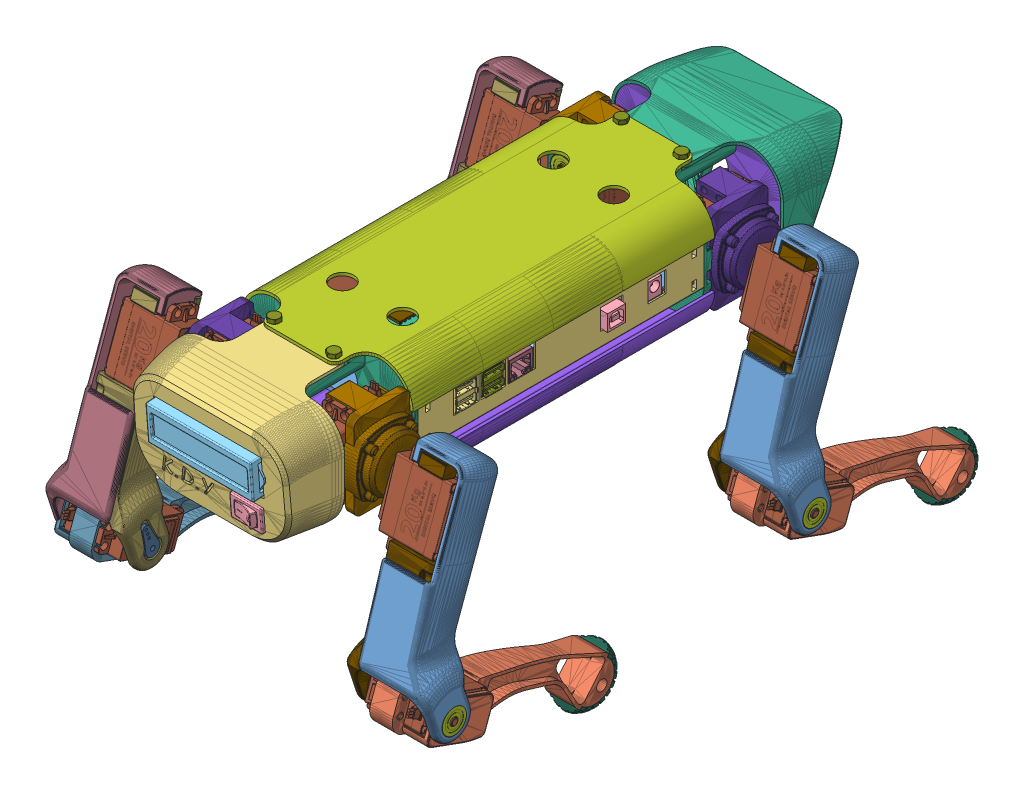
SolidWorks assembly Full Assembly [regular legs], configuration Default. Lengths in mm.
Overall size (257.32 212.52 418.73).
208 component instances, 46 part files, 86 mates.
Components (placement in the parent):
- Chase Assembly-1: Chase Assembly [Default] at (121.4756 142.8431 224.0299) size (112.8 70 292)
  - 1_2MCU_Plate-1: 1_2MCU_Plate [Default] at (22.3647 94.0168 229.1495) size (106 5.81 180)
  - 2_2MCU_Left_side_plate-1: 2_2MCU_Left_side_plate [Default] at (18.1147 57.0168 99.1495) x (1 0 0) z (0 -1 0) size (6.5 190 29)
  - 3_2MCU_Right_side_plate-1: 3_2MCU_Right_side_plate [Default] at (121.6147 57.0168 169.1495) x (-1 0 0) z (0 -1 0) size (6.5 190 29)
  - ArduinoMega-1: ArduinoMega [Default] at (70.5126 101.4678 88.5891) x (1 0 0) z (0 -1 0) size (107.95 53.42 12.95)
  - _Hex_Screws-1: _Hex_Screws [H M3x8] at (55.5647 101.4678 97.3157) x (-0.837169 0 -0.546944) z (-0.546944 0 0.837169) size (5.5 10 6.35) (hidden)
  - _Hex_Screws-2: _Hex_Screws [H M3x8] at (55.5647 101.4678 69.2995) x (0.837169 0 0.546944) z (0.546944 0 -0.837169) size (5.5 10 6.35) (hidden)
  - 4_M3_nut-1: 4_M3_nut [Default] at (55.5655 95.0168 69.2614) x (0.855198 0 0.518302) z (-0.518302 0 0.855198) size (6 2.34 5.2) (hidden)
  - 4_M3_nut-2: 4_M3_nut [Default] at (55.5332 95.0168 97.2415) x (-0.878773 0 0.47724) z (-0.47724 0 -0.878773) size (6 2.34 5.2) (hidden)
  - 12Channel PWM-1: 12Channel PWM [Default] at (79.9147 99.8168 132.7995) x (0 0 -1) z (1 0 0) size (25.4 7.55 66.7)
  - _M2_nut-1: _M2_nut [Default] at (51.9456 95.5168 142.2881) x (-0.74075 0 -0.671781) z (0 -1 0) size (4.67 4.62 1.63) (hidden)
  - _M2_nut-2: _M2_nut [Default] at (107.8452 93.9168 142.288) x (-0.738205 0 -0.674577) z (0 1 0) size (4.67 4.62 1.63) (hidden)
  - _M2_nut-3: _M2_nut [Default] at (107.8453 93.9168 123.488) x (-0.739008 0 -0.673697) z (0 1 0) size (4.67 4.62 1.63) (hidden)
  - _M2_nut-4: _M2_nut [Default] at (51.8785 93.9168 123.4273) x (-0.741456 0 -0.671001) z (0 1 0) size (4.67 4.62 1.63) (hidden)
  - _Hex_Screws-3: _Hex_Screws [H M2x8] at (51.9647 101.3268 142.1995) x (0.837169 0 0.546944) z (0.546944 0 -0.837169) size (4 9.4 4.62) (hidden)
  - _Hex_Screws-4: _Hex_Screws [H M2x8] at (107.8647 101.3268 123.3995) x (0.837169 0 0.546944) z (0.546944 0 -0.837169) size (4 9.4 4.62) (hidden)
  - _Hex_Screws-5: _Hex_Screws [H M2x8] at (51.9647 101.3268 123.3995) x (0.837169 0 0.546944) z (0.546944 0 -0.837169) size (4 9.4 4.62) (hidden)
  - _Hex_Screws-6: _Hex_Screws [H M2x8] at (107.8647 101.3268 142.1995) x (0.837169 0 0.546944) z (0.546944 0 -0.837169) size (4 9.4 4.62) (hidden)
  - _Hex_Screws-11: _Hex_Screws [H M2x8] at (40.2647 101.4168 153.7995) x (0.837169 0 0.546944) z (0.546944 0 -0.837169) size (4 9.4 4.62) (hidden)
  - _Hex_Screws-12: _Hex_Screws [H M2x8] at (98.2647 101.4068 153.7995) x (0.837169 0 0.546944) z (0.546944 0 -0.837169) size (4 9.4 4.62) (hidden)
  - _Hex_Screws-13: _Hex_Screws [H M2x8] at (40.2647 101.4068 202.7995) x (0.837169 0 0.546944) z (0.546944 0 -0.837169) size (4 9.4 4.62) (hidden)
  - _Hex_Screws-14: _Hex_Screws [H M2x8] at (98.2647 101.4168 202.7995) x (0.837169 0 0.546944) z (0.546944 0 -0.837169) size (4 9.4 4.62) (hidden)
  - _M2_nut-9: _M2_nut [Default] at (98.2838 93.9168 153.7109) x (-0.741324 0 -0.671147) z (0 1 0) size (4.67 4.62 1.63) (hidden)
  - _M2_nut-10: _M2_nut [Default] at (40.2838 93.9168 202.711) x (-0.74083 0 -0.671693) z (0 1 0) size (4.67 4.62 1.63) (hidden)
  - _M2_nut-11: _M2_nut [Default] at (98.2457 93.9168 202.8881) x (-0.741502 0 -0.670951) z (0 1 0) size (4.67 4.62 1.63) (hidden)
  - _M2_nut-12: _M2_nut [Default] at (40.3319 95.5168 153.8603) x (-0.741456 0 -0.671001) z (0 -1 0) size (4.67 4.62 1.63) (hidden)
  - Raspberry Pi 4 Model B-1: Raspberry Pi 4 Model B [Default] at (79.2647 100.6168 178.2995) size (89 19.92 58.4)
    - Raspberry Pi 4 Model B.STEP-1: Raspberry Pi 4 Model B.STEP [Default] at origin size (89 19.92 58.4)
      - PCB, RPi4ModelB.STEP-1: PCB, RPi4ModelB.STEP [Default] at origin size (85 1.6 56)
      - Broadcom BCM2711B0 CPU, RPi4ModelB.STEP-1: Broadcom BCM2711B0 CPU, RPi4ModelB.STEP [Default] at (-13.25 0.8 -4.5) size (15 2.3 15)
      - 2.54 mm DUPONT MALE PIN HEADER, POE, 2X2, RPi4ModelB.STEP-1: 2.54 mm DUPONT MALE PIN HEADER, POE, 2X2, RPi4ModelB.STEP [Default] at (19 0.8 -18.36) size (5.08 11.3 5.08)
      - 2.54 mm DUPONT MALE PIN HEADER, IO, 2X20, RPi4ModelB.STEP-1: 2.54 mm DUPONT MALE PIN HEADER, IO, 2X20, RPi4ModelB.STEP [Default] at (-10 0.8 -24.5) size (50.8 11.3 5.08)
      - Camera Connector, RPi4ModelB.STEP-1: Camera Connector, RPi4ModelB.STEP [Default] at (4 0.8 16.5) x (0 0 -1) z (1 0 0) size (22.4 5.68 5.07)
      - Microphone Plug, RPi4ModelB.STEP-1: Microphone Plug, RPi4ModelB.STEP [Default] at (11.5 0.8 21.65) size (7.23 7.55 15)
      - Display Connector, RPi4ModelB.STEP-1: Display Connector, RPi4ModelB.STEP [Default] at (-38.5 0.8 0) x (0 0 1) z (-1 0 0) size (22.4 5.68 5.07)
      - Gigabit Ethernet Port, RPi4ModelB.STEP-1: Gigabit Ethernet Port, RPi4ModelB.STEP [Default] at (45.5 7.55 -17.75) x (0 0 -1) z (1 0 0) size (16.33 17.24 21.6)
      - Female Micro HDMI Connector, RPi4ModelB.STEP-1: Female Micro HDMI Connector, RPi4ModelB.STEP [Default] at (-3 0.8 27.3875) size (6.5 3.51 7.5)
      - Female Micro HDMI Connector, RPi4ModelB.STEP-2: Female Micro HDMI Connector, RPi4ModelB.STEP [Default] at (-16.5 0.8 27.3875) size (6.5 3.51 7.5)
      - Female USB Type C Connector, RPi4ModelB.STEP-1: Female USB Type C Connector, RPi4ModelB.STEP [Default] at (-31.3 0.8 26.5419) size (8.94 3.96 7.9)
      - 2X USB3.0 PORTS, RPi4ModelB.STEP-1: 2X USB3.0 PORTS, RPi4ModelB.STEP [Default] at (37.07 0.8 1) size (17.48 19.42 15.69)
      - 91D77 D9WHV 778K, 4 GB LPDDR4 SDRAM, RPi4ModelB.STEP-1: 91D77 D9WHV 778K, 4 GB LPDDR4 SDRAM, RPi4ModelB.STEP [Default] at (2.25 0.8 -4.5) size (10 0.8 14.5)
      - Cypress CYW43455 Wireless Module Cover, RPi4ModelB.STEP-1: Cypress CYW43455 Wireless Module Cover, RPi4ModelB.STEP [Default] at (-30.5 0.8 -14.5) size (11 1.6 13)
      - SD Card Slot, RPi4ModelB.STEP-1: SD Card Slot, RPi4ModelB.STEP [Default] at (-35.3 -0.8 0) x (0 0 -1) z (-1 0 0) size (11.95 1.45 11.4)
      - VIA VL805 PCIe USB 3.0 controller, RPi4ModelB.STEP-1: VIA VL805 PCIe USB 3.0 controller, RPi4ModelB.STEP [Default] at (17.5 0.8 4) size (8.8 0.8 8.8)
      - 2X USB2.0 PORTS, RPi4ModelB.STEP-1: 2X USB2.0 PORTS, RPi4ModelB.STEP [Default] at (37.065 0.65 19) size (17.87 19.17 15.35)
      - Broadcom BCM54213PE Gigabit Ethernet Transceiver, RPi4ModelB.STEP-1: Broadcom BCM54213PE Gigabit Ethernet Transceiver, RPi4ModelB.STEP [Default] at (16.5 0.8 -10) size (6.8 1 6.8)
      - MxL7704 Universal PMIC, RPi4ModelB.STEP-1: MxL7704 Universal PMIC, RPi4ModelB.STEP [Default] at (-32.5 0.8 16) size (5.4 0.8 5.4)
  - 6_Front_shoulder_mg-1: 6_Front_shoulder_mg [Default] at (124.8647 139.0168 39.1495) x (-1 0 0) z (0 -1 0) size (110 51 70)
  - 6_Front_shoulder_mg-2: 6_Front_shoulder_mg [Default] at (14.8647 139.0168 229.1495) x (1 0 0) z (0 -1 0) size (110 51 70)
  - _Hex_Screws-15: _Hex_Screws [H M3x12] at (18.2198 96.9886 231.1495) x (1 0 0) z (0 1 0) size (5.5 14 6.35) (hidden)
  - _Hex_Screws-16: _Hex_Screws [H M3x12] at (121.5159 97.0038 231.1495) x (1 0 0) z (0 1 0) size (5.5 14 6.35) (hidden)
  - _Hex_Screws-17: _Hex_Screws [H M3x12] at (18.2375 115.9459 231.1495) x (-0.998805 0.048869 0) z (-0.048869 -0.998805 0) size (5.5 14 6.35) (hidden)
  - _Hex_Screws-18: _Hex_Screws [H M3x12] at (18.1956 96.9701 37.1495) x (0.969974 0.243208 0) z (0.243208 -0.969974 0) size (5.5 14 6.35) (hidden)
  - _Hex_Screws-19: _Hex_Screws [H M3x12] at (18.1916 115.9399 37.1495) x (1 0 0) z (0 -1 0) size (5.5 14 6.35) (hidden)
  - _Hex_Screws-20: _Hex_Screws [H M3x12] at (121.5019 115.9701 231.1495) x (0.105991 0.994367 0) z (-0.994367 0.105991 0) size (5.5 14 6.35) (hidden)
  - _Hex_Screws-21: _Hex_Screws [H M3x12] at (121.6489 115.9342 37.1495) x (1 0 0) z (0 -1 0) size (5.5 14 6.35) (hidden)
  - _Hex_Screws-22: _Hex_Screws [H M3x12] at (121.6691 96.9226 37.1495) x (1 0 0) z (0 -1 0) size (5.5 14 6.35) (hidden)
  - 4_M3_nut-4: 4_M3_nut [Default] at (18.0647 96.9149 222.1495) x (1 0 0) z (0 -1 0) size (6 2.34 5.2) (hidden)
  - 4_M3_nut-5: 4_M3_nut [Default] at (18.0647 115.9149 222.1495) x (1 0 0) z (0 -1 0) size (6 2.34 5.2) (hidden)
  - 4_M3_nut-6: 4_M3_nut [Default] at (121.6647 96.9149 222.1495) x (1 0 0) z (0 -1 0) size (6 2.34 5.2) (hidden)
  - 4_M3_nut-7: 4_M3_nut [Default] at (121.6647 115.9149 222.1495) x (1 0 0) z (0 -1 0) size (6 2.34 5.2) (hidden)
  - 4_M3_nut-8: 4_M3_nut [Default] at (18.0647 115.9149 46.1495) x (0.5 0.866025 0) z (-0.866025 0.5 0) size (6 2.34 5.2) (hidden)
  - 4_M3_nut-9: 4_M3_nut [Default] at (18.0647 96.9149 44.1495) x (1 0 0) z (0 -1 0) size (6 2.34 5.2) (hidden)
  - 4_M3_nut-10: 4_M3_nut [Default] at (121.6647 96.9149 44.1495) x (1 0 0) z (0 -1 0) size (6 2.34 5.2) (hidden)
  - 4_M3_nut-11: 4_M3_nut [Default] at (121.6647 115.9149 46.1495) x (0.5 -0.866025 0) z (0.866025 0.5 0) size (6 2.34 5.2) (hidden)
  - F625ZZ Ball Bearing-1: F625ZZ Ball Bearing [Default] at (31.004 104.9515 234.1495) x (1 0 0) z (0 0 1) size (18 18 5)
  - F625ZZ Ball Bearing-2: F625ZZ Ball Bearing [Default] at (104.9018 120.0403 234.1495) x (-0.879341 -0.476193 0) z (0 0 1) size (18 18 5)
  - F625ZZ Ball Bearing-3: F625ZZ Ball Bearing [Default] at (30.2307 104.9537 34.1495) x (-0.995136 0.098516 0) z (0 0 -1) size (18 18 5)
  - F625ZZ Ball Bearing-4: F625ZZ Ball Bearing [Default] at (111.8008 105.7118 34.1495) x (-0.923728 -0.383049 0) z (0 0 -1) size (18 18 5)
- Front Legs-1: Front Legs [Default] at (233.7989 374.0539 299.7914) x (-1 0 0) z (0 -1 0) size (257.32 168.18 205.82)
  - 7_Rear_shoulder-2: 7_Rear_shoulder [Default] at (-12.5249 87.612 92.1876) size (110 5 66)
  - Left Leg Assembly-1: Left Leg Assembly [Default] at (86.5165 30.9423 148.2853) size (111.25 167.25 201.66)
    - Left_arm_joint_mg-1: Left_arm_joint_mg [Default] at (-15.0415 19.5698 -40.5977) size (37.5 46 56.5)
    - Servohorn-1: Servohorn [4 Prong] at (19.6585 29.8198 -20.3477) x (0 -0.592234 0.805766) z (-1 0 0) size (31.8 31.8 2.24)
    - Servo Motor-1: Servo Motor [Default] at (-5.0415 40.5698 -30.0977) size (20.1 45.99 55.6)
    - Servohorn-2: Servohorn [Default] at (-5.0415 60.9698 -30.0977) x (0.506689 0 -0.862129) z (0 -1 0) size (28.18 31.8 2.24)
    - Servo Motor-2: Servo Motor [Default] at (38.0585 29.8198 -20.3477) x (0 0.939693 0.34202) z (0 -0.34202 0.939693) size (20.1 45.99 55.6)
    - Left_arm_mg-1: Left_arm_mg [Default] at (38.0585 42.7737 -26.7003) x (0 -0.939693 -0.34202) z (0 -0.34202 0.939693) size (38.24 39.8 137.4)
    - SM_Left_arm_cover-1: SM_Left_arm_cover [Default] at (38.2585 50.3364 -32.5645) x (0 -0.939693 -0.34202) z (0 -0.34202 0.939693) size (41.16 45 143.55)
    - F625ZZ Ball Bearing-1: F625ZZ Ball Bearing [Default] at (78.2585 -1.6568 83.7617) x (0 -0.070361 0.997522) z (-1 0 0) size (18 18 5)
    - Servohorn-3: Servohorn [1 Prong] at (28.0585 6.3719 84.4796) x (0 0.893193 -0.449674) z (1 0 0) size (9.55 20.65 2.24)
    - Left_wrist_mg-1: Left_wrist_mg [Default] at (18.4585 0.3781 71.7095) x (0 0.939693 0.34202) z (0 -0.34202 0.939693) size (149.99 36.9 30)
    - foot-1: foot [Default] at (48.4585 115.3593 124.2008) x (0 0.642788 -0.766044) z (0 -0.766044 -0.642788) size (38.32 20 19.41)
    - Servo Motor-3: Servo Motor [Default] at (48.4585 6.3719 84.4796) x (0 0.34202 -0.939693) z (0 0.939693 0.34202) size (20.1 45.99 55.6)
    - _Hex_Screws-1: _Hex_Screws [H M4x20] at (-0.0415 43.7698 3.9023) x (-0.837169 0 -0.546944) z (-0.546944 0 0.837169) size (7 22.8 8.08) (hidden)
    - _Hex_Screws-2: _Hex_Screws [H M4x20] at (-10.0415 43.7698 -44.0977) x (-0.837169 0 -0.546944) z (-0.546944 0 0.837169) size (7 22.8 8.08) (hidden)
    - _Hex_Screws-3: _Hex_Screws [H M4x20] at (-10.0415 43.7698 3.9023) x (-0.837169 0 -0.546944) z (-0.546944 0 0.837169) size (7 22.8 8.08) (hidden)
    - _Hex_Screws-4: _Hex_Screws [H M4x20] at (-0.0415 43.7698 -44.0977) x (-0.837169 0 -0.546944) z (-0.546944 0 0.837169) size (7 22.8 8.08) (hidden)
    - _Hex_Screws-5: _Hex_Screws [H M4x20] at (34.8585 22.8895 13.3119) x (0 0.825172 -0.564882) z (0 -0.564882 -0.825172) size (7 22.8 8.08) (hidden)
    - _Hex_Screws-6: _Hex_Screws [H M4x20] at (34.8585 13.4926 9.8917) x (0 0.825172 -0.564882) z (0 -0.564882 -0.825172) size (7 22.8 8.08) (hidden)
    - _Hex_Screws-7: _Hex_Screws [H M4x20] at (34.8585 39.3065 -31.7933) x (0 0.802845 -0.596188) z (0 -0.596188 -0.802845) size (7 22.8 8.08) (hidden)
    - _Hex_Screws-8: _Hex_Screws [H M4x20] at (34.8585 29.9096 -35.2135) x (0 -0.944714 0.327896) z (0 0.327896 0.944714) size (7 22.8 8.08) (hidden)
    - _Hex_Screws-9: _Hex_Screws [H M4x20] at (45.2585 40.0315 91.4099) x (0 0.825172 -0.564882) z (0 -0.564882 -0.825172) size (7 22.8 8.08) (hidden)
    - _Hex_Screws-10: _Hex_Screws [H M4x20] at (45.2585 36.6113 100.8068) x (0 0.825172 -0.564882) z (0 -0.564882 -0.825172) size (7 22.8 8.08) (hidden)
    - _Hex_Screws-11: _Hex_Screws [H M4x20] at (45.2585 -5.0737 74.9929) x (0 0.825172 -0.564882) z (0 -0.564882 -0.825172) size (7 22.8 8.08) (hidden)
    - _Hex_Screws-12: _Hex_Screws [H M4x20] at (45.2585 -8.4939 84.3898) x (0 0.825172 -0.564882) z (0 -0.564882 -0.825172) size (7 22.8 8.08) (hidden)
    - _Hex_Screws-13: _Hex_Screws [H M3x16] at (62.9617 14.9879 55.4881) x (0.992954 0.04053 -0.111356) z (-0.118503 0.33961 -0.933071) size (5.5 18 6.35)
  - Right Leg Assembly-1: Right Leg Assembly [Default] at (19.1728 32.9715 132.7261) size (64.22 167.45 199.81)
    - Right_arm_joint_mg-1: Right_arm_joint_mg [Default] at (24.2858 18.5405 -25.0321) size (37.5 46 56.5)
    - Servohorn-1: Servohorn [4 Prong] at (-38.4142 28.7905 -4.7821) x (0 0.715501 0.698611) z (-1 0 0) size (31.8 31.8 2.24)
    - Servo Motor-1: Servo Motor [Default] at (-15.7142 38.5405 -14.5321) size (20.1 45.99 55.6)
    - Servohorn-2: Servohorn [Default] at (-15.7142 58.9405 -14.5321) x (-0.99999 0 0.00451) z (0 -1 0) size (28.18 31.8 2.24)
    - Right_arm_mg-1: Right_arm_mg [Default] at (-8.8142 41.6076 -10.7588) x (0 -0.939693 -0.34202) z (0 -0.34202 0.939693) size (38.24 39.8 137.4)
    - SM_Right_arm_cover-1: SM_Right_arm_cover [Default] at (-48.6142 49.0427 -16.5661) x (0 -0.939693 -0.34202) z (0 -0.34202 0.939693) size (41.16 45 143.55)
    - F625ZZ Ball Bearing-1: F625ZZ Ball Bearing [Default] at (-98.6142 -2.6723 100.0196) x (0 0.0383 -0.999266) z (1 0 0) size (18 18 5)
    - Servohorn-3: Servohorn [1 Prong] at (-48.8142 5.2058 100.4211) x (0 -0.953491 0.301422) z (-1 0 0) size (9.55 20.65 2.24)
    - Servo Motor-2: Servo Motor [Default] at (-67.7142 5.2058 100.4211) x (0 -0.34202 0.939693) z (0 0.939693 0.34202) size (20.1 45.99 55.6)
    - Servo Motor-3: Servo Motor [Default] at (-58.8142 28.7905 -4.7821) x (0 -0.939693 -0.34202) z (0 -0.34202 0.939693) size (20.1 45.99 55.6)
    - Right_wrist_mg-1: Right_wrist_mg [Default] at (-67.7142 -0.7709 87.604) x (0 0.939693 0.34202) z (0 -0.34202 0.939693) size (149.99 36.9 30)
    - foot-1: foot [Default] at (-67.7142 114.2242 140.0873) x (0 -0.656061 0.754708) z (0 -0.754708 -0.656061) size (38.32 20 19.41)
    - _Hex_Screws-1: _Hex_Screws [H M4x20] at (-20.7142 41.7405 19.4679) x (-0.837169 0 -0.546944) z (-0.546944 0 0.837169) size (7 22.8 8.08) (hidden)
    - _Hex_Screws-2: _Hex_Screws [H M4x20] at (-10.7142 41.7405 -28.5321) x (-0.837169 0 -0.546944) z (-0.546944 0 0.837169) size (7 22.8 8.08) (hidden)
    - _Hex_Screws-3: _Hex_Screws [H M4x20] at (-10.7142 41.7405 19.4679) x (-0.99108 0 -0.133267) z (-0.133267 0 0.99108) size (7 22.8 8.08) (hidden)
    - _Hex_Screws-4: _Hex_Screws [H M4x20] at (-20.7142 41.7405 -28.5321) x (0.837169 0 0.546944) z (0.546944 0 -0.837169) size (7 22.8 8.08) (hidden)
    - _Hex_Screws-5: _Hex_Screws [H M4x20] at (-55.6142 28.8803 -19.6479) x (0 0.085299 -0.996355) z (0 0.996355 0.085299) size (7 22.8 8.08) (hidden)
    - _Hex_Screws-8: _Hex_Screws [H M4x20] at (-55.6142 12.4633 25.4573) x (0 -0.381849 0.924225) z (0 -0.924225 -0.381849) size (7 22.8 8.08) (hidden)
    - _Hex_Screws-9: _Hex_Screws [H M4x20] at (-55.6142 21.8603 28.8775) x (0 -0.381849 0.924225) z (0 -0.924225 -0.381849) size (7 22.8 8.08) (hidden)
    - _Hex_Screws-10: _Hex_Screws [H M4x20] at (-64.5142 -9.66 100.3313) x (0 -0.381849 0.924225) z (0 -0.924225 -0.381849) size (7 22.8 8.08) (hidden)
    - _Hex_Screws-11: _Hex_Screws [H M4x20] at (-64.5142 38.8655 107.3514) x (0 -0.381849 0.924225) z (0 -0.924225 -0.381849) size (7 22.8 8.08) (hidden)
    - _Hex_Screws-12: _Hex_Screws [H M4x20] at (-64.5142 -6.2398 90.9344) x (0 -0.381849 0.924225) z (0 -0.924225 -0.381849) size (7 22.8 8.08) (hidden)
    - _Hex_Screws-14: _Hex_Screws [H M4x20] at (-64.5142 35.4453 116.7483) x (0 -0.381849 0.924225) z (0 -0.924225 -0.381849) size (7 22.8 8.08) (hidden)
    - _Hex_Screws-15: _Hex_Screws [H M4x20] at (-55.6142 38.2772 -16.2277) x (0 0.381849 -0.924225) z (0 0.924225 0.381849) size (7 22.8 8.08) (hidden)
    - _Hex_Screws-19: _Hex_Screws [H M3x16] at (-83.8911 13.8209 71.432) x (0.19625 0.335369 -0.921419) z (-0.980554 0.067122 -0.184415) size (5.5 18 6.35)
- Back Legs-1: Back Legs [Default] at (148.8652 374.0475 416.5673) x (1 0 0) z (0 -1 0) size (257.32 168.18 205.82)
  - 7_Rear_shoulder-2: 7_Rear_shoulder [Default] at (-12.5249 87.612 92.1876) size (110 5 66)
  - Back Left Leg Assembly-1: Back Left Leg Assembly [Default] at (86.5165 30.9423 148.2853) size (109.75 167.45 202.02)
    - Left_arm_joint_mg-1: Left_arm_joint_mg [Default] at (-15.0415 19.5698 -40.5977) size (37.5 46 56.5)
    - Servohorn-1: Servohorn [4 Prong] at (19.6585 29.8198 -20.3477) x (0 -0.698611 0.715501) z (-1 0 0) size (31.8 31.8 2.24)
    - Servo Motor-1: Servo Motor [Default] at (-5.0415 40.5698 -30.0977) size (20.1 45.99 55.6)
    - Servohorn-2: Servohorn [Default] at (-5.0415 60.9698 -30.0977) x (0.506689 0 -0.862129) z (0 -1 0) size (28.18 31.8 2.24)
    - _Hex_Screws-1: _Hex_Screws [H M4x20] at (-0.0415 43.7698 3.9023) x (-0.837169 0 -0.546944) z (-0.546944 0 0.837169) size (7 22.8 8.08) (hidden)
    - _Hex_Screws-2: _Hex_Screws [H M4x20] at (-10.0415 43.7698 -44.0977) x (-0.837169 0 -0.546944) z (-0.546944 0 0.837169) size (7 22.8 8.08) (hidden)
    - _Hex_Screws-3: _Hex_Screws [H M4x20] at (-10.0415 43.7698 3.9023) x (-0.837169 0 -0.546944) z (-0.546944 0 0.837169) size (7 22.8 8.08) (hidden)
    - _Hex_Screws-4: _Hex_Screws [H M4x20] at (-0.0415 43.7698 -44.0977) x (-0.837169 0 -0.546944) z (-0.546944 0 0.837169) size (7 22.8 8.08) (hidden)
    - _Hex_Screws-14: _Hex_Screws [H M3x16] at (63.1355 44.7893 55.8664) x (-0.19625 -0.335369 -0.921419) z (0.980554 -0.067122 -0.184415) size (5.5 18 6.35)
    - _Hex_Screws-15: _Hex_Screws [H M4x20] at (34.8585 20.333 -31.7933) x (0 -0.381849 -0.924225) z (0 -0.924225 0.381849) size (7 22.8 8.08) (hidden)
    - _Hex_Screws-16: _Hex_Screws [H M4x20] at (43.7585 64.85 75.3688) x (0 0.381849 0.924225) z (0 0.924225 -0.381849) size (7 22.8 8.08) (hidden)
    - _Hex_Screws-17: _Hex_Screws [H M4x20] at (43.7585 23.165 101.1827) x (0 0.381849 0.924225) z (0 0.924225 -0.381849) size (7 22.8 8.08) (hidden)
    - _Hex_Screws-18: _Hex_Screws [H M4x20] at (43.7585 19.7448 91.7857) x (0 0.381849 0.924225) z (0 0.924225 -0.381849) size (7 22.8 8.08) (hidden)
    - _Hex_Screws-19: _Hex_Screws [H M4x20] at (43.7585 68.2702 84.7657) x (0 0.381849 0.924225) z (0 0.924225 -0.381849) size (7 22.8 8.08) (hidden)
    - _Hex_Screws-20: _Hex_Screws [H M4x20] at (34.8585 36.75 13.3119) x (0 0.381849 0.924225) z (0 0.924225 -0.381849) size (7 22.8 8.08) (hidden)
    - _Hex_Screws-21: _Hex_Screws [H M4x20] at (34.8585 46.1469 9.8917) x (0 0.381849 0.924225) z (0 0.924225 -0.381849) size (7 22.8 8.08) (hidden)
    - _Hex_Screws-22: _Hex_Screws [H M4x20] at (34.8585 29.7299 -35.2135) x (0 -0.085299 -0.996355) z (0 -0.996355 0.085299) size (7 22.8 8.08) (hidden)
    - foot-2: foot [Default] at (46.9585 -55.614 124.5217) x (0 0.656061 0.754708) z (0 0.754708 -0.656061) size (38.32 20 19.41)
    - Right_wrist_mg-1: Right_wrist_mg [Default] at (46.9585 59.3812 72.0384) x (0 -0.939693 0.34202) z (0 0.34202 0.939693) size (149.99 36.9 30)
    - Servo Motor-4: Servo Motor [Default] at (38.0585 29.8198 -20.3477) x (0 0.939693 -0.34202) z (0 0.34202 0.939693) size (20.1 45.99 55.6)
    - Servo Motor-5: Servo Motor [Default] at (46.9585 53.4044 84.8555) x (0 0.34202 0.939693) z (0 -0.939693 0.34202) size (20.1 45.99 55.6)
    - Servohorn-4: Servohorn [1 Prong] at (28.0585 53.4044 84.8555) x (0 0.953491 0.301422) z (1 0 0) size (9.55 20.65 2.24)
    - F625ZZ Ball Bearing-2: F625ZZ Ball Bearing [Default] at (77.8585 61.2825 84.454) x (0 -0.0383 -0.999266) z (-1 0 0) size (18 18 5)
    - SM_Right_arm_cover-1: SM_Right_arm_cover [Default] at (27.8586 9.5676 -32.1317) x (0 0.939693 -0.34202) z (0 0.34202 0.939693) size (41.16 45 143.55)
    - Right_arm_mg-1: Right_arm_mg [Default] at (-11.9415 17.0026 -26.3245) x (0 0.939693 -0.34202) z (0 0.34202 0.939693) size (38.24 39.8 137.4)
  - Back Right Leg Assembly-1: Back Right Leg Assembly [Default] at (19.1728 32.9715 132.7261) size (104.56 167.25 200.75)
    - Right_arm_joint_mg-1: Right_arm_joint_mg [Default] at (24.2858 18.5405 -25.0321) size (37.5 46 56.5)
    - Servohorn-1: Servohorn [4 Prong] at (-38.4142 28.7905 -4.7821) x (0 0.715501 0.698611) z (-1 0 0) size (31.8 31.8 2.24)
    - Servo Motor-1: Servo Motor [Default] at (-15.7142 38.5405 -14.5321) size (20.1 45.99 55.6)
    - Servohorn-2: Servohorn [Default] at (-15.7142 58.9405 -14.5321) x (-0.99999 0 0.00451) z (0 -1 0) size (28.18 31.8 2.24)
    - _Hex_Screws-1: _Hex_Screws [H M4x20] at (-20.7142 41.7405 19.4679) x (-0.837169 0 -0.546944) z (-0.546944 0 0.837169) size (7 22.8 8.08) (hidden)
    - _Hex_Screws-2: _Hex_Screws [H M4x20] at (-10.7142 41.7405 -28.5321) x (-0.837169 0 -0.546944) z (-0.546944 0 0.837169) size (7 22.8 8.08) (hidden)
    - _Hex_Screws-3: _Hex_Screws [H M4x20] at (-10.7142 41.7405 19.4679) x (-0.99108 0 -0.133267) z (-0.133267 0 0.99108) size (7 22.8 8.08) (hidden)
    - _Hex_Screws-4: _Hex_Screws [H M4x20] at (-20.7142 41.7405 -28.5321) x (0.837169 0 0.546944) z (0.546944 0 -0.837169) size (7 22.8 8.08) (hidden)
    - _Hex_Screws-20: _Hex_Screws [H M3x16] at (-83.7173 43.6223 71.0537) x (0.992954 0.04053 0.111356) z (-0.118503 0.33961 0.933071) size (5.5 18 6.35) (hidden)
    - _Hex_Screws-21: _Hex_Screws [H M4x20] at (-66.0142 67.1041 99.9555) x (0 0.149128 -0.988818) z (0 0.988818 0.149128) size (7 22.8 8.08) (hidden)
    - _Hex_Screws-22: _Hex_Screws [H M4x20] at (-66.0142 63.6839 90.5585) x (0 -0.837169 0.546944) z (0 -0.546944 -0.837169) size (7 22.8 8.08) (hidden)
    - _Hex_Screws-23: _Hex_Screws [H M4x20] at (-66.0142 21.9989 116.3724) x (0 -0.837169 0.546944) z (0 -0.546944 -0.837169) size (7 22.8 8.08) (hidden)
    - _Hex_Screws-24: _Hex_Screws [H M4x20] at (-66.0142 18.5787 106.9755) x (0 -0.837169 0.546944) z (0 -0.546944 -0.837169) size (7 22.8 8.08) (hidden)
    - _Hex_Screws-25: _Hex_Screws [H M4x20] at (-55.6142 28.7007 -19.6479) x (0 0.663788 -0.747921) z (0 0.747921 0.663788) size (7 22.8 8.08) (hidden)
    - _Hex_Screws-26: _Hex_Screws [H M4x20] at (-55.6142 19.3037 -16.2277) x (0 -0.857577 0.514355) z (0 -0.514355 -0.857577) size (7 22.8 8.08) (hidden)
    - _Hex_Screws-27: _Hex_Screws [H M4x20] at (-55.6142 45.1176 25.4573) x (0 -0.837169 0.546944) z (0 -0.546944 -0.837169) size (7 22.8 8.08) (hidden)
    - _Hex_Screws-28: _Hex_Screws [H M4x20] at (-55.6142 35.7207 28.8775) x (0 -0.837169 0.546944) z (0 -0.546944 -0.837169) size (7 22.8 8.08) (hidden)
    - Servo Motor-4: Servo Motor [Default] at (-69.2142 52.2383 100.0453) x (0 -0.34202 -0.939693) z (0 -0.939693 0.34202) size (20.1 45.99 55.6)
    - foot-2: foot [Default] at (-69.2142 -56.7491 139.7664) x (0 -0.642788 -0.766044) z (0 0.766044 -0.642788) size (38.32 20 19.41)
    - Left_wrist_mg-1: Left_wrist_mg [Default] at (-39.2142 58.2322 87.2751) x (0 -0.939693 0.34202) z (0 0.34202 0.939693) size (149.99 36.9 30)
    - Servohorn-4: Servohorn [1 Prong] at (-48.8142 52.2383 100.0453) x (0 -0.947083 -0.320989) z (-1 0 0) size (9.55 20.65 2.24)
    - F625ZZ Ball Bearing-2: F625ZZ Ball Bearing [Default] at (-99.0142 54.8139 92.2998) x (0 0.948801 0.315873) z (1 0 0) size (18 18 5)
    - SM_Left_arm_cover-1: SM_Left_arm_cover [Default] at (-59.0142 8.2739 -16.9989) x (0 0.939693 -0.34202) z (0 0.34202 0.939693) size (41.16 45 143.55)
    - Left_arm_mg-1: Left_arm_mg [Default] at (-58.8142 15.8365 -11.1347) x (0 0.939693 -0.34202) z (0 0.34202 0.939693) size (38.24 39.8 137.4)
    - Servo Motor-5: Servo Motor [Default] at (-58.8142 28.7905 -4.7821) x (0 -0.939693 0.34202) z (0 0.34202 0.939693) size (20.1 45.99 55.6)
- Back Assembly-1: Back Assembly [Default] at (224.5857 241.5151 483.7838) x (0 -1 0) z (0 0 -1) size (70 114 75.42)
  - SM_Rear_cover_mg-1: SM_Rear_cover_mg [Default] at (-38.2447 -23.7546 -24.8955) size (70 114 69.85)
  - rocker switch 1-1: rocker switch 1 [test] at (14.374 8.6954 -53.0846) x (-0.997054 0 -0.076697) z (0.076697 0 -0.997054) size (15 21 21.16)
  - LCDScreen-1: LCDScreen [Default] at (-11.6228 33.6204 -49.4804) x (0 -1 0) z (0.997054 0 0.076697) size (79.38 18.26 34.92)
- SM_Front_cover_mg-1: SM_Front_cover_mg [Default] at (134.3403 281.7599 237.6794) x (0 0 -1) z (0 -1 0) size (92.81 114 70)
- _Hex_Screws-1: _Hex_Screws [H M3x16] at (171.2241 274.9622 210.1794) x (0.859899 0.510465 0) z (0.510465 -0.859899 0) size (5.5 18 6.35) (hidden)
- _Hex_Screws-2: _Hex_Screws [H M3x16] at (186.2241 218.9622 210.1794) x (0.972339 -0.233574 0) z (-0.233574 -0.972339 0) size (5.5 18 6.35) (hidden)
- _Hex_Screws-3: _Hex_Screws [H M3x16] at (196.4229 218.9578 210.1794) x (0.270134 -0.962823 0) z (-0.962823 -0.270134 0) size (5.5 18 6.35) (hidden)
- _Hex_Screws-4: _Hex_Screws [H M3x16] at (211.4201 274.9364 210.1794) x (0.993065 -0.117567 0) z (-0.117567 -0.993065 0) size (5.5 18 6.35) (hidden)
- _Hex_Screws-5: _Hex_Screws [H M3x16] at (171.4531 274.8132 506.1794) x (0.646462 -0.762947 0) z (0.762947 0.646462 0) size (5.5 18 6.35) (hidden)
- _Hex_Screws-6: _Hex_Screws [H M3x16] at (196.4112 218.9827 506.1794) x (0.945209 0.326467 0) z (-0.326467 0.945209 0) size (5.5 18 6.35) (hidden)
- _Hex_Screws-7: _Hex_Screws [H M3x16] at (211.3403 275.0016 506.1794) x (0.48223 -0.876045 0) z (0.876045 0.48223 0) size (5.5 18 6.35) (hidden)
- _Hex_Screws-8: _Hex_Screws [H M3x16] at (186.4998 218.9259 506.1794) x (-0.065426 0.997857 0) z (-0.997857 -0.065426 0) size (5.5 18 6.35) (hidden)
- 4_M3_nut-1: 4_M3_nut [Default] at (196.1403 219.2618 498.1794) x (0.5 0.866025 0) z (-0.866025 0.5 0) size (6 2.34 5.2) (hidden)
- 4_M3_nut-2: 4_M3_nut [Default] at (186.5403 219.2618 498.1794) x (0.5 0.866025 0) z (-0.866025 0.5 0) size (6 2.34 5.2) (hidden)
- 4_M3_nut-3: 4_M3_nut [Default] at (171.1403 275.2618 498.1794) x (1 0 0) z (0 1 0) size (6 2.34 5.2) (hidden)
- 4_M3_nut-4: 4_M3_nut [Default] at (211.1403 275.2618 498.1794) x (0.5 0.866025 0) z (-0.866025 0.5 0) size (6 2.34 5.2) (hidden)
- 4_M3_nut-5: 4_M3_nut [Default] at (196.5403 219.2618 218.1794) x (1 0 0) z (0 -1 0) size (6 2.34 5.2) (hidden)
- 4_M3_nut-6: 4_M3_nut [Default] at (211.1403 275.2618 218.1794) x (0.5 -0.866025 0) z (-0.866025 -0.5 0) size (6 2.34 5.2) (hidden)
- 4_M3_nut-7: 4_M3_nut [Default] at (186.5403 219.2618 218.1794) x (0.5 -0.866025 0) z (-0.866025 -0.5 0) size (6 2.34 5.2) (hidden)
- 4_M3_nut-8: 4_M3_nut [Default] at (171.5403 275.2618 218.1794) x (1 0 0) z (0 -1 0) size (6 2.34 5.2) (hidden)
- Custom_Top_cover_mg-1: Custom_Top_cover_mg [Default] at (134.3403 159.7599 508.1794) x (0 0 -1) z (1 0 0) size (240 21.5 113.99)
- Custom_Bottom_cover_mg-1: Custom_Bottom_cover_mg [Default] at (248.3403 333.7599 508.1794) x (0 0 -1) z (-1 0 0) size (240 21.5 113.99)
- _Hex_Screws-9: _Hex_Screws [H M4x12] at (211.3403 283.7599 243.1794) x (-0.837169 0 -0.546944) z (-0.546944 0 0.837169) size (7 14.8 8.08)
- _Hex_Screws-10: _Hex_Screws [H M4x12] at (171.3403 283.7599 243.1794) x (-0.837169 0 -0.546944) z (-0.546944 0 0.837169) size (7 14.8 8.08)
- _Hex_Screws-11: _Hex_Screws [H M4x12] at (210.5302 283.7599 473.0727) x (-0.459347 0 -0.888257) z (-0.888257 0 0.459347) size (7 14.8 8.08)
- _Hex_Screws-12: _Hex_Screws [H M4x12] at (170.7987 283.7599 472.8667) x (0.643444 0 -0.765493) z (-0.765493 0 -0.643444) size (7 14.8 8.08)
- _Hex_Screws-13: _Hex_Screws [H M4x12] at (196.3403 209.7599 243.1794) size (7 14.8 8.08)
- _Hex_Screws-14: _Hex_Screws [H M4x12] at (186.3403 209.7599 243.1794) size (7 14.8 8.08)
- _Hex_Screws-15: _Hex_Screws [H M4x12] at (196.3403 209.7599 473.1794) size (7 14.8 8.08)
- _Hex_Screws-16: _Hex_Screws [H M4x12] at (186.3403 209.7599 473.1794) size (7 14.8 8.08)
Mates (geometry in assembly coordinates):
- Concentric2: concentric aligned: circle of Chase Assembly-1/6_Front_shoulder_mg-2; circle of Front Legs-1/7_Rear_shoulder-2
- Parallel1: parallel aligned: plane of Chase Assembly-1/6_Front_shoulder_mg-2 through (136.3403 279.8599 453.1794) normal (0 1 0); plane of Front Legs-1/7_Rear_shoulder-2 through (246.3238 279.8663 212.1794) normal (0 1 0)
- Coincident14: coincident anti-aligned: plane of Chase Assembly-1/6_Front_shoulder_mg-2 through (136.3403 279.8599 453.1794) normal (0 1 0); plane of Back Assembly-1/SM_Rear_cover_mg-1 through (248.3403 279.8599 508.6794) normal (0 -1 0)
- Distance1: distance = 1 mm anti-aligned: plane of Chase Assembly-1/6_Front_shoulder_mg-2 through (136.3403 281.8599 467.6794) normal (0 0 1); plane of Back Assembly-1/SM_Rear_cover_mg-1 through (248.3403 279.7599 468.6794) normal (0 0 -1)
- Coincident16: coincident aligned: plane of Chase Assembly-1/6_Front_shoulder_mg-2 through (216.3403 281.8599 453.1794) normal (1 0 0); plane of Back Assembly-1/SM_Rear_cover_mg-1 through (216.3403 279.7599 508.6794) normal (1 0 0)
- Coincident17: coincident anti-aligned: plane of Chase Assembly-1/6_Front_shoulder_mg-1 through (246.3403 279.8599 263.1794) normal (0 1 0); plane of SM_Front_cover_mg-1 through (134.3403 279.8599 237.6794) normal (0 -1 0)
- Coincident19: coincident aligned: plane of Chase Assembly-1/6_Front_shoulder_mg-1 through (166.3403 281.8599 263.1794) normal (-1 0 0); plane of SM_Front_cover_mg-1 through (166.3403 281.7599 237.6794) normal (-1 0 0)
- Distance2: distance = 1 mm anti-aligned: plane of SM_Front_cover_mg-1 through (134.3403 281.7599 247.6794) normal (0 0 1); plane of Chase Assembly-1/6_Front_shoulder_mg-1 through (246.3403 281.8599 248.6794) normal (0 0 -1)
- Coincident21: coincident: line of Chase Assembly-1/6_Front_shoulder_mg-1 through (171.7544 276.4053 212.1794) axis (1 0 0); plane of Front Legs-1/7_Rear_shoulder-2 through (246.3238 281.8663 212.1794) normal (0 0 1)
- Coincident22: coincident anti-aligned: plane of Chase Assembly-1/6_Front_shoulder_mg-2 through (136.3403 281.8599 504.1794) normal (0 0 1); plane of Back Legs-1/7_Rear_shoulder-2 through (136.3403 281.8599 504.1794) normal (0 0 -1)
- Coincident23: coincident aligned: plane of Chase Assembly-1/6_Front_shoulder_mg-2 through (136.3403 279.8599 453.1794) normal (0 1 0); plane of Back Legs-1/7_Rear_shoulder-2 through (136.3403 279.8599 504.1794) normal (0 1 0)
- Coincident24: coincident aligned: plane of Chase Assembly-1/6_Front_shoulder_mg-2 through (136.3403 281.8599 453.1794) normal (-1 0 0); plane of Back Legs-1/7_Rear_shoulder-2 through (136.3403 281.8599 504.1794) normal (-1 0 0)
- Coincident28: coincident anti-aligned: plane of Front Legs-1/7_Rear_shoulder-2 through (246.3238 281.8663 210.1794) normal (0 0 -1); plane of _Hex_Screws-1 through (171.2241 274.9622 210.1794) normal (0 0 1)
- Coincident29: coincident anti-aligned: plane of Front Legs-1/7_Rear_shoulder-2 through (246.3238 281.8663 210.1794) normal (0 0 -1); plane of _Hex_Screws-4 through (211.4201 274.9364 210.1794) normal (0 0 1)
- Coincident30: coincident anti-aligned: plane of Front Legs-1/7_Rear_shoulder-2 through (246.3238 281.8663 210.1794) normal (0 0 -1); plane of _Hex_Screws-2 through (186.2241 218.9622 210.1794) normal (0 0 1)
- Coincident31: coincident anti-aligned: plane of Front Legs-1/7_Rear_shoulder-2 through (246.3238 281.8663 210.1794) normal (0 0 -1); plane of _Hex_Screws-3 through (196.4229 218.9578 210.1794) normal (0 0 1)
- Tangent8: tangent anti-aligned: plane of Chase Assembly-1/6_Front_shoulder_mg-1 through (253.4339 227.976 263.1794) normal (0.13052 -0.991446 0); cylinder of _Hex_Screws-3 through (196.4229 218.9578 226.1794) axis (0 0 -1) radius 1.5
- Tangent9: tangent anti-aligned: plane of Front Legs-1/7_Rear_shoulder-2 through (206.9007 287.0561 212.1794) normal (-0.991446 0.13052 0); cylinder of _Hex_Screws-3 through (196.4229 218.9578 226.1794) axis (0 0 -1) radius 1.5
- Tangent10: tangent anti-aligned: plane of Chase Assembly-1/6_Front_shoulder_mg-1 through (237.3728 213.7417 263.1794) normal (-0.13052 -0.991446 0); cylinder of _Hex_Screws-2 through (186.2241 218.9622 226.1794) axis (0 0 -1) radius 1.5
- Tangent11: tangent anti-aligned: plane of Front Legs-1/7_Rear_shoulder-2 through (177.6208 272.8218 212.1794) normal (0.991446 0.13052 0); cylinder of _Hex_Screws-2 through (186.2241 218.9622 226.1794) axis (0 0 -1) radius 1.5
- Tangent12: tangent anti-aligned: plane of Chase Assembly-1/6_Front_shoulder_mg-1 through (245.0452 272.0225 263.1794) normal (-0.130526 -0.991445 0); cylinder of _Hex_Screws-4 through (211.4201 274.9364 226.1794) axis (0 0 -1) radius 1.5
- Tangent13: tangent anti-aligned: plane of Front Legs-1/7_Rear_shoulder-2 through (214.3986 286.0691 212.1794) normal (-0.991446 0.13052 0); cylinder of _Hex_Screws-4 through (211.4201 274.9364 226.1794) axis (0 0 -1) radius 1.5
- Tangent14: tangent anti-aligned: cylinder of _Hex_Screws-1 through (171.2241 274.9622 226.1794) axis (0 0 -1) radius 1.5; plane of Chase Assembly-1/6_Front_shoulder_mg-1 through (244.3637 266.8462 263.1794) normal (-0.130526 -0.991445 0)
- Tangent15: tangent anti-aligned: plane of Front Legs-1/7_Rear_shoulder-2 through (170.1231 271.8334 212.1794) normal (0.991443 0.130537 0); cylinder of _Hex_Screws-1 through (171.2241 274.9622 226.1794) axis (0 0 -1) radius 1.5
- Coincident32: coincident anti-aligned: plane of Back Legs-1/7_Rear_shoulder-2 through (136.3403 281.8599 506.1794) normal (0 0 1); circle of _Hex_Screws-5
- Coincident33: coincident anti-aligned: plane of Back Legs-1/7_Rear_shoulder-2 through (136.3403 281.8599 506.1794) normal (0 0 1); plane of _Hex_Screws-7 through (211.3403 275.0016 506.1794) normal (0 0 -1)
- Coincident34: coincident aligned: plane of Back Legs-1/7_Rear_shoulder-2 through (136.3403 281.8599 506.1794) normal (0 0 1); circle of _Hex_Screws-8
- Coincident35: coincident anti-aligned: plane of Back Legs-1/7_Rear_shoulder-2 through (136.3403 281.8599 506.1794) normal (0 0 1); plane of _Hex_Screws-6 through (196.4112 218.9827 506.1794) normal (0 0 -1)
- Tangent16: tangent anti-aligned: plane of Back Legs-1/7_Rear_shoulder-2 through (166.7948 208.3384 504.1794) normal (0.382693 -0.923876 0); cylinder of _Hex_Screws-6 through (196.4112 218.9827 490.1794) axis (0 0 1) radius 1.5
- Tangent17: tangent anti-aligned: plane of Back Legs-1/7_Rear_shoulder-2 through (188.7385 288.7579 504.1794) normal (-0.991446 -0.13052 0); cylinder of _Hex_Screws-6 through (196.4112 218.9827 490.1794) axis (0 0 1) radius 1.5
- Tangent18: tangent anti-aligned: plane of Back Legs-1/7_Rear_shoulder-2 through (199.4962 233.3995 504.1794) normal (-0.793359 0.608754 0); cylinder of _Hex_Screws-8 through (186.4998 218.9259 490.1794) axis (0 0 1) radius 1.5
- Tangent19: tangent anti-aligned: plane of Chase Assembly-1/6_Front_shoulder_mg-2 through (129.2467 227.976 453.1794) normal (-0.13052 -0.991446 0); cylinder of _Hex_Screws-8 through (186.4998 218.9259 490.1794) axis (0 0 1) radius 1.5
- Tangent20: tangent anti-aligned: plane of Chase Assembly-1/6_Front_shoulder_mg-2 through (165.2053 293.8162 453.1794) normal (-0.923879 -0.382684 0); cylinder of _Hex_Screws-5 through (171.4531 274.8132 490.1794) axis (0 0 1) radius 1.5
- Tangent21: tangent anti-aligned: plane of Chase Assembly-1/6_Front_shoulder_mg-2 through (144.5479 262.0451 453.1794) normal (-0.382684 0.923879 0); cylinder of _Hex_Screws-5 through (171.4531 274.8132 490.1794) axis (0 0 1) radius 1.5
- Tangent22: tangent anti-aligned: plane of Chase Assembly-1/6_Front_shoulder_mg-2 through (181.4243 316.4535 453.1794) normal (-0.793358 -0.608756 0); cylinder of _Hex_Screws-7 through (211.3403 275.0016 490.1794) axis (0 0 1) radius 1.5
- Tangent23: tangent anti-aligned: plane of Chase Assembly-1/6_Front_shoulder_mg-2 through (185.6677 244.009 453.1794) normal (0.793349 -0.608767 0); cylinder of _Hex_Screws-7 through (211.3403 275.0016 490.1794) axis (0 0 1) radius 1.5
- Coincident36: coincident anti-aligned: plane of Chase Assembly-1/6_Front_shoulder_mg-2 through (136.3403 281.8599 496.1794) normal (0 0 1); plane of 4_M3_nut-2 through (186.5403 219.2618 496.1794) normal (0 0 -1)
- Coincident37: coincident anti-aligned: plane of Chase Assembly-1/6_Front_shoulder_mg-2 through (136.3403 281.8599 496.1794) normal (0 0 1); plane of 4_M3_nut-1 through (196.1403 219.2618 496.1794) normal (0 0 -1)
- Coincident38: coincident anti-aligned: plane of Chase Assembly-1/6_Front_shoulder_mg-2 through (136.3403 281.8599 496.1794) normal (0 0 1); plane of 4_M3_nut-4 through (211.1403 275.2618 496.1794) normal (0 0 -1)
- Coincident39: coincident anti-aligned: plane of Chase Assembly-1/6_Front_shoulder_mg-2 through (136.3403 281.8599 496.1794) normal (0 0 1); plane of 4_M3_nut-3 through (171.1403 275.2618 496.1794) normal (0 0 -1)
- Distance3: distance = 2 mm aligned: plane of Chase Assembly-1/6_Front_shoulder_mg-2 through (136.3403 279.8599 453.1794) normal (0 1 0); plane of 4_M3_nut-3 through (169.6403 277.8599 496.1794) normal (0 1 0)
- Coincident41: coincident: plane of Chase Assembly-1/6_Front_shoulder_mg-2 through (174.1403 281.8599 453.1794) normal (-1 0 0); line of 4_M3_nut-3 through (174.1403 275.2618 496.4114) axis (0 0 1)
- Distance4: distance = 2 mm aligned: plane of 4_M3_nut-4 through (209.6403 277.8599 496.1794) normal (0 1 0); plane of Chase Assembly-1/6_Front_shoulder_mg-2 through (136.3403 279.8599 453.1794) normal (0 1 0)
- Coincident43: coincident: plane of Chase Assembly-1/6_Front_shoulder_mg-2 through (214.1403 281.8599 453.1794) normal (-1 0 0); line of 4_M3_nut-4 through (214.1403 275.2618 496.4114) axis (0 0 1)
- Distance5: distance = 2 mm aligned: plane of 4_M3_nut-2 through (185.0403 221.8599 496.1794) normal (0 1 0); plane of Chase Assembly-1/6_Front_shoulder_mg-2 through (136.3403 223.8599 453.1794) normal (0 1 0)
- Coincident45: coincident: plane of Chase Assembly-1/6_Front_shoulder_mg-2 through (183.5403 281.8599 453.1794) normal (1 0 0); line of 4_M3_nut-2 through (183.5403 219.2618 496.4114) axis (0 0 1)
- Distance6: distance = 2 mm aligned: plane of 4_M3_nut-1 through (194.6403 221.8599 496.1794) normal (0 1 0); plane of Chase Assembly-1/6_Front_shoulder_mg-2 through (136.3403 223.8599 453.1794) normal (0 1 0)
- Coincident47: coincident: plane of Chase Assembly-1/6_Front_shoulder_mg-2 through (199.1403 281.8599 453.1794) normal (-1 0 0); line of 4_M3_nut-1 through (199.1403 219.2618 496.4114) axis (0 0 1)
- Coincident48: coincident anti-aligned: plane of Chase Assembly-1/6_Front_shoulder_mg-1 through (246.3403 281.8599 220.1794) normal (0 0 -1); plane of 4_M3_nut-6 through (211.1403 275.2618 220.1794) normal (0 0 1)
- Coincident49: coincident anti-aligned: plane of Chase Assembly-1/6_Front_shoulder_mg-1 through (246.3403 281.8599 220.1794) normal (0 0 -1); plane of 4_M3_nut-8 through (171.5403 275.2618 220.1794) normal (0 0 1)
- Coincident50: coincident anti-aligned: plane of Chase Assembly-1/6_Front_shoulder_mg-1 through (246.3403 281.8599 220.1794) normal (0 0 -1); plane of 4_M3_nut-5 through (196.5403 219.2618 220.1794) normal (0 0 1)
- Coincident51: coincident anti-aligned: plane of Chase Assembly-1/6_Front_shoulder_mg-1 through (246.3403 281.8599 220.1794) normal (0 0 -1); plane of 4_M3_nut-7 through (186.5403 219.2618 220.1794) normal (0 0 1)
- Distance7: distance = 2 mm aligned: plane of 4_M3_nut-7 through (188.0403 221.8599 220.1794) normal (0 1 0); plane of Chase Assembly-1/6_Front_shoulder_mg-1 through (246.3403 223.8599 263.1794) normal (0 1 0)
- Coincident53: coincident: plane of Chase Assembly-1/6_Front_shoulder_mg-1 through (183.5403 281.8599 263.1794) normal (1 0 0); line of 4_M3_nut-7 through (183.5403 219.2618 219.9473) axis (0 0 -1)
- Distance8: distance = 2 mm aligned: plane of Chase Assembly-1/6_Front_shoulder_mg-1 through (246.3403 223.8599 263.1794) normal (0 1 0); plane of 4_M3_nut-5 through (198.0403 221.8599 220.1794) normal (0 1 0)
- Coincident55: coincident: plane of Chase Assembly-1/6_Front_shoulder_mg-1 through (193.5403 281.8599 263.1794) normal (1 0 0); line of 4_M3_nut-5 through (193.5403 219.2618 219.9473) axis (0 0 -1)
- Distance9: distance = 2 mm aligned: plane of 4_M3_nut-8 through (173.0403 277.8599 220.1794) normal (0 1 0); plane of Chase Assembly-1/6_Front_shoulder_mg-1 through (246.3403 279.8599 263.1794) normal (0 1 0)
- Coincident57: coincident: plane of Chase Assembly-1/6_Front_shoulder_mg-1 through (168.5403 281.8599 263.1794) normal (1 0 0); line of 4_M3_nut-8 through (168.5403 275.2618 219.9473) axis (0 0 -1)
- Distance10: distance = 2 mm aligned: plane of 4_M3_nut-6 through (212.6403 277.8599 220.1794) normal (0 1 0); plane of Chase Assembly-1/6_Front_shoulder_mg-1 through (246.3403 279.8599 263.1794) normal (0 1 0)
- Coincident59: coincident: plane of Chase Assembly-1/6_Front_shoulder_mg-1 through (214.1403 281.8599 263.1794) normal (-1 0 0); line of 4_M3_nut-6 through (214.1403 275.2618 219.9473) axis (0 0 -1)
- Coincident60: coincident anti-aligned: plane of SM_Front_cover_mg-1 through (134.3403 281.7599 237.6794) normal (0 1 0); plane of Custom_Top_cover_mg-1 through (134.3403 281.7599 508.1794) normal (0 -1 0)
- Parallel3: parallel anti-aligned: line of Back Assembly-1/SM_Rear_cover_mg-1 through (171.3403 281.7599 468.6794) axis (1 0 0); line of Custom_Top_cover_mg-1 through (211.3403 283.7599 478.1794) axis (-1 0 0)
- Coincident62: coincident aligned: plane of Chase Assembly-1/6_Front_shoulder_mg-1 through (246.3403 281.8599 258.1794) normal (0 0 -1); plane of Custom_Top_cover_mg-1 through (226.257 261.6746 258.1794) normal (0 0 -1)
- Coincident64: coincident aligned: plane of Back Assembly-1/SM_Rear_cover_mg-1 through (216.3403 279.7599 508.6794) normal (1 0 0); plane of Custom_Top_cover_mg-1 through (216.3403 159.7599 508.1794) normal (1 0 0)
- Coincident65: coincident anti-aligned: plane of SM_Front_cover_mg-1 through (134.3403 211.7599 237.6794) normal (0 -1 0); plane of Custom_Bottom_cover_mg-1 through (248.3403 211.7599 508.1794) normal (0 1 0)
- Parallel5: parallel aligned: line of SM_Front_cover_mg-1 through (186.3403 211.7599 247.6794) axis (1 0 0); line of Custom_Bottom_cover_mg-1 through (186.3403 209.7599 478.1794) axis (1 0 0)
- Coincident67: coincident aligned: plane of Chase Assembly-1/6_Front_shoulder_mg-2 through (136.3403 281.8599 458.1794) normal (0 0 1); plane of Custom_Bottom_cover_mg-1 through (248.3403 333.7599 458.1794) normal (0 0 1)
- Coincident68: coincident aligned: plane of Back Assembly-1/SM_Rear_cover_mg-1 through (181.3403 279.7599 508.6794) normal (-1 0 0); plane of Custom_Bottom_cover_mg-1 through (181.3403 211.7599 468.1794) normal (-1 0 0)
- Coincident69: coincident anti-aligned: plane of Custom_Top_cover_mg-1 through (134.3403 283.7599 508.1794) normal (0 1 0); plane of _Hex_Screws-10 through (171.3403 283.7599 243.1794) normal (0 -1 0)
- Coincident70: coincident anti-aligned: plane of Custom_Top_cover_mg-1 through (134.3403 283.7599 508.1794) normal (0 1 0); plane of _Hex_Screws-9 through (211.3403 283.7599 243.1794) normal (0 -1 0)
- Coincident71: coincident anti-aligned: plane of Custom_Top_cover_mg-1 through (134.3403 283.7599 508.1794) normal (0 1 0); plane of _Hex_Screws-11 through (210.5302 283.7599 473.0727) normal (0 -1 0)
- Coincident72: coincident anti-aligned: plane of Custom_Top_cover_mg-1 through (134.3403 283.7599 508.1794) normal (0 1 0); plane of _Hex_Screws-12 through (170.7987 283.7599 472.8667) normal (0 -1 0)
- Tangent24: tangent anti-aligned: plane of Custom_Top_cover_mg-1 through (170.0403 249.2599 470.9277) normal (0.608759 0 0.793355); cylinder of _Hex_Screws-12 through (170.7987 271.7599 472.8667) axis (0 1 0) radius 2
- Tangent25: tangent anti-aligned: plane of Custom_Top_cover_mg-1 through (168.8289 249.2599 472.5064) normal (0.991445 0 0.130524); cylinder of _Hex_Screws-12 through (170.7987 271.7599 472.8667) axis (0 1 0) radius 2
- Tangent26: tangent anti-aligned: plane of Custom_Top_cover_mg-1 through (210.0403 249.2599 470.9277) normal (0.608761 0 0.793353); cylinder of _Hex_Screws-11 through (210.5302 271.7599 473.0727) axis (0 1 0) radius 2
- Tangent27: tangent anti-aligned: plane of Custom_Top_cover_mg-1 through (209.0886 249.2599 474.4794) normal (0.793355 0 -0.608759); cylinder of _Hex_Screws-11 through (210.5302 271.7599 473.0727) axis (0 1 0) radius 2
- Concentric3: concentric aligned: cylinder of Custom_Top_cover_mg-1 through (211.3403 281.7599 243.1794) axis (0 1 0) radius 2.5778; cylinder of _Hex_Screws-9 through (211.3403 271.7599 243.1794) axis (0 1 0) radius 2
- Concentric4: concentric aligned: cylinder of Custom_Top_cover_mg-1 through (171.3403 281.7599 243.1794) axis (0 1 0) radius 2.5778; cylinder of _Hex_Screws-10 through (171.3403 271.7599 243.1794) axis (0 1 0) radius 2
- Coincident74: coincident anti-aligned: plane of Custom_Bottom_cover_mg-1 through (248.3403 209.7599 508.1794) normal (0 -1 0); plane of _Hex_Screws-14 through (186.3403 209.7599 243.1794) normal (0 1 0)
- Coincident75: coincident anti-aligned: plane of Custom_Bottom_cover_mg-1 through (248.3403 209.7599 508.1794) normal (0 -1 0); plane of _Hex_Screws-15 through (196.3403 209.7599 473.1794) normal (0 1 0)
- Coincident76: coincident anti-aligned: plane of Custom_Bottom_cover_mg-1 through (248.3403 209.7599 508.1794) normal (0 -1 0); plane of _Hex_Screws-13 through (196.3403 209.7599 243.1794) normal (0 1 0)
- Coincident77: coincident anti-aligned: plane of Custom_Bottom_cover_mg-1 through (248.3403 209.7599 508.1794) normal (0 -1 0); plane of _Hex_Screws-16 through (186.3403 209.7599 473.1794) normal (0 1 0)
- Concentric5: concentric aligned: cylinder of Custom_Bottom_cover_mg-1 through (186.3403 211.7599 243.1794) axis (0 -1 0) radius 2.5778; cylinder of _Hex_Screws-14 through (186.3403 221.7599 243.1794) axis (0 -1 0) radius 2
- Concentric6: concentric aligned: circle of Custom_Bottom_cover_mg-1; cylinder of _Hex_Screws-13 through (196.3403 221.7599 243.1794) axis (0 -1 0) radius 2
- Concentric7: concentric aligned: cylinder of Custom_Bottom_cover_mg-1 through (186.3403 211.7599 473.1794) axis (0 -1 0) radius 2.5778; cylinder of _Hex_Screws-16 through (186.3403 221.7599 473.1794) axis (0 -1 0) radius 2
- Concentric8: concentric aligned: cylinder of Custom_Bottom_cover_mg-1 through (196.3403 211.7599 473.1794) axis (0 -1 0) radius 2.5778; cylinder of _Hex_Screws-15 through (196.3403 221.7599 473.1794) axis (0 -1 0) radius 2
